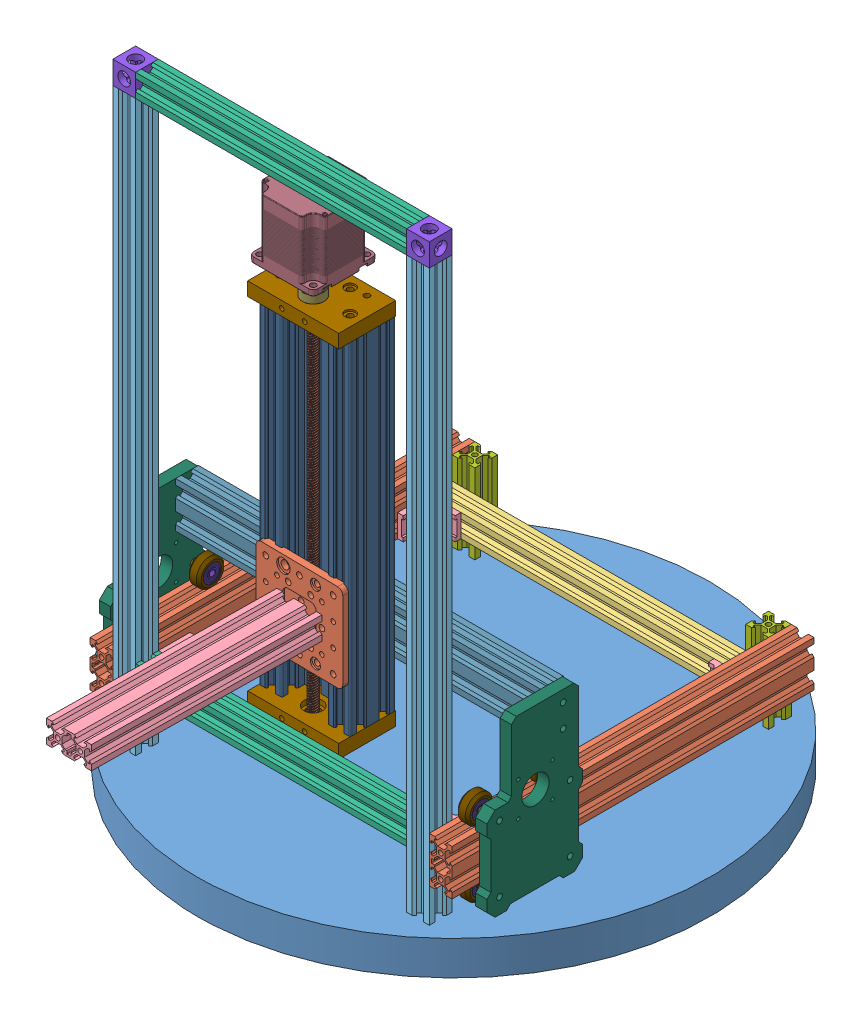
SolidWorks assembly Main, configuration Predeterminado. Lengths in mm.
Overall size (450 550 553.32).
74 component instances, 23 part files, 11 mates.
Components (placement in the parent):
- Base-1: Base [Predeterminado] at (-4.6545 -30.3598 450) size (450 30 450)
- XFrame-1: XFrame [Predeterminado] at (-136.0419 47.8198 132.7398) x (1 0 -0.000004) z (0.000004 0 1) size (318 520 318)
  - XBosch2040-1: XBosch2040 [Predeterminado] at (-28.3648 1.8204 159) size (20 40 318)
  - XBosch2020-3: XBosch2020 [Predeterminado] at (-8.3648 1.8204 457) x (0 0 -1) z (1 0 0) size (20 20 278)
  - XBosch2040-3: XBosch2040 [Predeterminado] at (269.6352 1.8204 159) size (20 40 318)
  - XBosch2020-4: XBosch2020 [Predeterminado] at (-8.3648 1.8204 199) x (0 0 -1) z (1 0 0) size (20 20 278)
  - 20X28.step-1: 20X28.step [Predeterminado] at (-8.3648 -8.1796 423.1) x (0 1 0) z (1 0 0) size (20 29.3 29.3)
  - 20X28.step-2: 20X28.step [Predeterminado] at (255.7352 -8.1796 437) x (0 1 0) z (0 0 -1) size (20 29.3 29.3)
  - 20X28.step-5: 20X28.step [Predeterminado] at (269.6352 -8.1796 212.9) x (0 1 0) z (-1 0 0) size (20 29.3 29.3)
  - 20X28.step-6: 20X28.step [Predeterminado] at (-8.3648 -8.1796 212.9) x (0 -1 0) z (1 0 0) size (20 29.3 29.3)
  - BaseKinectBosch2020-1: BaseKinectBosch2020 [Predeterminado] at (249.6352 -48.1796 477) x (0 0 -1) z (0 1 0) size (20 20 500)
  - BaseKinectBosch2020-3: BaseKinectBosch2020 [Predeterminado] at (-8.3648 -48.1796 477) x (0 0 -1) z (0 1 0) size (20 20 500)
  - SupportKinectBosch2020-2: SupportKinectBosch2020 [Predeterminado] at (11.6352 21.8204 477) x (0 0 -1) z (1 0 0) size (20 20 238)
  - SupportKinectBosch2020-3: SupportKinectBosch2020 [Predeterminado] at (11.6352 471.8204 477) x (0 0 -1) z (1 0 0) size (20 20 238)
  - SBaseKinectBosch2020-1: SBaseKinectBosch2020 [Predeterminado] at (-8.3648 21.8204 179) x (1 0 0) z (0 -1 0) size (20 20 70)
  - SBaseKinectBosch2020-2: SBaseKinectBosch2020 [Predeterminado] at (249.6352 21.8204 179) x (1 0 0) z (0 -1 0) size (20 20 70)
  - 2020CubeConnector.stp-1: 2020CubeConnector.stp [Predeterminado] at (-8.3648 451.8204 477) size (20 20 20)
  - 2020CubeConnector.stp-2: 2020CubeConnector.stp [Predeterminado] at (269.6352 451.8204 477) x (0 0 -1) z (1 0 0) size (20 20 20)
- LinearActuator-1: LinearActuator [Predeterminado] at (-0.8488 42.2282 481.3447) x (1 0 -0.000004) z (0.000004 0 1) size (80 409.44 60.6)
  - C-BeamEnd-2: C-BeamEnd [Predeterminado] at (-11.3983 29.7078 77.0996) x (1 0 0) z (0 0 -1) size (80 12 50)
  - C-Beam300-2: C-Beam300 [Predeterminado] at (-11.3983 329.7078 72.0996) x (-1 0 0) z (0 -1 0) size (80 40 300)
  - ScrewAxisZ-1: ScrewAxisZ [Default] at (-11.3983 17.7078 84.4996) x (0.069055 0 -0.997613) z (0 -1 0) size (8.33 8.33 405.47)
  - C-BeamEnd-3: C-BeamEnd [Predeterminado] at (-11.3983 329.7078 77.0996) x (-1 0 0) z (0 0 -1) size (80 12 50)
  - Coupler 6.35-8mm-1: Coupler 6.35-8mm [Default] at (-11.3983 354.2078 84.4996) x (0.045113 0 -0.998982) z (0 1 0) size (19.34 19.34 25)
  - Nema 23-1: Nema 23 [Default] at (-11.3983 424.3078 84.4996) x (-1 0 0) z (0 -1 0) size (56.4 59.4 76.6)
- YAxis-1: YAxis [Predeterminado] at (-525.5801 128.1994 508.9368) x (-0.000004 0 -1) z (1 0 -0.000004) size (90.84 144.12 340.6)
  - YBosch2040-1: YBosch2040 [Predeterminado] at (-24.5098 3.6408 360) size (20 40 320.6)
  - AxisY-Carrier-1: AxisY-Carrier [Predeterminado] at (-39.5098 -77.3592 350) size (84.07 143.54 10)
  - AxisY-Carrier-2: AxisY-Carrier [Predeterminado] at (-39.5098 -77.3592 680.6) size (84.07 143.54 10)
  - INSERTO_M5x0,8x6-2: INSERTO_M5x0,8x6 [Valor predeterminado] at (-70.5098 -48.3592 360) x (0.849028 0.528347 0) z (0.528347 -0.849028 0) size (7 6.95 6.99)
  - INSERTO_M5x0,8x6-3: INSERTO_M5x0,8x6 [Valor predeterminado] at (-8.5098 -48.3592 360) x (0 1 0) z (1 0 0) size (7 6.95 6.99)
  - INSERTO_M5x0,8x6-4: INSERTO_M5x0,8x6 [Valor predeterminado] at (-70.5098 -106.3592 360) x (0 1 0) z (1 0 0) size (7 6.95 6.99)
  - INSERTO_M5x0,8x6-5: INSERTO_M5x0,8x6 [Valor predeterminado] at (-8.5098 -106.3592 360) x (0 1 0) z (1 0 0) size (7 6.95 6.99)
  - INSERTO_M5x0,8x6-6: INSERTO_M5x0,8x6 [Valor predeterminado] at (-8.5098 -48.3592 674.6) x (0 1 0) z (1 0 0) size (7 6.95 6.99)
  - INSERTO_M5x0,8x6-7: INSERTO_M5x0,8x6 [Valor predeterminado] at (-70.5098 -48.3592 674.6) x (0.840532 0.541762 0) z (0.541762 -0.840532 0) size (7 6.95 6.99)
  - INSERTO_M5x0,8x6-8: INSERTO_M5x0,8x6 [Valor predeterminado] at (-8.5098 -106.3592 674.6) x (0 1 0) z (1 0 0) size (7 6.95 6.99)
  - INSERTO_M5x0,8x6-9: INSERTO_M5x0,8x6 [Valor predeterminado] at (-70.5098 -106.3592 674.6) x (0 1 0) z (1 0 0) size (7 6.95 6.99)
  - nylon-pulley-wheel-625zz.step-1: nylon-pulley-wheel-625zz.step [Predeterminado] at (-70.5098 -106.3592 669.4) x (0 0 -1) z (-0.999997 0.00242 0) size (10.4 24 24)
    - SKF_625_2Z v1.step-1: SKF_625_2Z v1.step [Predeterminado] at (-5.2 0 0) size (5 16 16)
    - Roldana V Nylon.step-1: Roldana V Nylon.step [Predeterminado] at origin size (10.4 24 24)
    - SKF_625_2Z v1 (1).step-1: SKF_625_2Z v1 (1).step [Predeterminado] at (5.2 0 0) x (-1 0 0) z (0 0 1) size (5 16 16)
  - nylon-pulley-wheel-625zz.step-2: nylon-pulley-wheel-625zz.step [Predeterminado] at (-70.5098 -48.3592 669.4) x (0 0 -1) z (1 0 0) size (10.4 24 24)
    - SKF_625_2Z v1.step-1: SKF_625_2Z v1.step [Predeterminado] at (-5.2 0 0) size (5 16 16)
    - Roldana V Nylon.step-1: Roldana V Nylon.step [Predeterminado] at origin size (10.4 24 24)
    - SKF_625_2Z v1 (1).step-1: SKF_625_2Z v1 (1).step [Predeterminado] at (5.2 0 0) x (-1 0 0) z (0 0 1) size (5 16 16)
  - nylon-pulley-wheel-625zz.step-3: nylon-pulley-wheel-625zz.step [Predeterminado] at (-8.5098 -48.3592 669.4) x (0 0 -1) z (0.968642 0.248459 0) size (10.4 24 24)
    - SKF_625_2Z v1.step-1: SKF_625_2Z v1.step [Predeterminado] at (-5.2 0 0) size (5 16 16)
    - Roldana V Nylon.step-1: Roldana V Nylon.step [Predeterminado] at origin size (10.4 24 24)
    - SKF_625_2Z v1 (1).step-1: SKF_625_2Z v1 (1).step [Predeterminado] at (5.2 0 0) x (-1 0 0) z (0 0 1) size (5 16 16)
  - nylon-pulley-wheel-625zz.step-4: nylon-pulley-wheel-625zz.step [Predeterminado] at (-8.5098 -106.3592 669.4) x (0 0 -1) z (0.999938 -0.011103 0) size (10.4 24 24)
    - SKF_625_2Z v1.step-1: SKF_625_2Z v1.step [Predeterminado] at (-5.2 0 0) size (5 16 16)
    - Roldana V Nylon.step-1: Roldana V Nylon.step [Predeterminado] at origin size (10.4 24 24)
    - SKF_625_2Z v1 (1).step-1: SKF_625_2Z v1 (1).step [Predeterminado] at (5.2 0 0) x (-1 0 0) z (0 0 1) size (5 16 16)
  - nylon-pulley-wheel-625zz.step-5: nylon-pulley-wheel-625zz.step [Predeterminado] at (-8.5098 -106.3592 371.2) x (0 0 -1) z (1 0 0) size (10.4 24 24)
    - SKF_625_2Z v1.step-1: SKF_625_2Z v1.step [Predeterminado] at (-5.2 0 0) size (5 16 16)
    - Roldana V Nylon.step-1: Roldana V Nylon.step [Predeterminado] at origin size (10.4 24 24)
    - SKF_625_2Z v1 (1).step-1: SKF_625_2Z v1 (1).step [Predeterminado] at (5.2 0 0) x (-1 0 0) z (0 0 1) size (5 16 16)
  - nylon-pulley-wheel-625zz.step-6: nylon-pulley-wheel-625zz.step [Predeterminado] at (-70.5098 -106.3592 371.2) x (0 0 -1) z (0.980573 0.196154 0) size (10.4 24 24)
    - SKF_625_2Z v1.step-1: SKF_625_2Z v1.step [Predeterminado] at (-5.2 0 0) size (5 16 16)
    - Roldana V Nylon.step-1: Roldana V Nylon.step [Predeterminado] at origin size (10.4 24 24)
    - SKF_625_2Z v1 (1).step-1: SKF_625_2Z v1 (1).step [Predeterminado] at (5.2 0 0) x (-1 0 0) z (0 0 1) size (5 16 16)
  - nylon-pulley-wheel-625zz.step-7: nylon-pulley-wheel-625zz.step [Predeterminado] at (-70.5098 -48.3592 371.2) x (0 0 -1) z (1 0 0) size (10.4 24 24)
    - SKF_625_2Z v1.step-1: SKF_625_2Z v1.step [Predeterminado] at (-5.2 0 0) size (5 16 16)
    - Roldana V Nylon.step-1: Roldana V Nylon.step [Predeterminado] at origin size (10.4 24 24)
    - SKF_625_2Z v1 (1).step-1: SKF_625_2Z v1 (1).step [Predeterminado] at (5.2 0 0) x (-1 0 0) z (0 0 1) size (5 16 16)
  - nylon-pulley-wheel-625zz.step-8: nylon-pulley-wheel-625zz.step [Predeterminado] at (-8.5098 -48.3592 371.2) x (0 0 -1) z (0.965283 -0.261208 0) size (10.4 24 24)
    - SKF_625_2Z v1.step-1: SKF_625_2Z v1.step [Predeterminado] at (-5.2 0 0) size (5 16 16)
    - Roldana V Nylon.step-1: Roldana V Nylon.step [Predeterminado] at origin size (10.4 24 24)
    - SKF_625_2Z v1 (1).step-1: SKF_625_2Z v1 (1).step [Predeterminado] at (5.2 0 0) x (-1 0 0) z (0 0 1) size (5 16 16)
- Arm-1: Arm [Predeterminado] at (-11.8566 145.5398 494.6935) x (0.999919 0 0.012739) z (-0.012739 0 0.999919) size (77.15 77.15 218)
  - C-BeamPlate-1: C-BeamPlate [Predeterminado] at (0.5163 1.4458 77.15) x (0 1 0) z (0 0 1) size (77.15 77.15 6)
  - Anti-BacklashBlock-1: Anti-BacklashBlock [Predeterminado] at (0.5163 -2.0542 65.15) x (0 -1 0) z (-1 0 0) size (33 12 34)
  - ZBosch2040-1: ZBosch2040 [Predeterminado] at (0.5163 11.4458 83.15) x (0 -1 0) z (0 0 1) size (20 40 200)
- CilinderForY-1: CilinderForY [Predeterminado] at (-159.5796 59.5227 607.7399) x (-0.000002 -0.902624 -0.43043) z (1 0 -0.000004) size (4 4 1.35)
Mates (geometry in assembly coordinates):
- Bloquear1: lock: unknown of Base-1; unknown of XFrame-1/XBosch2020-1
- Coincidente1: coincident anti-aligned: plane of LinearActuator-1/C-Beam300-2 through (-17.6668 371.936 533.4444) normal (-0.000004 0 -1); plane of YAxis-1/YBosch2040-1 through (155.02 131.8402 533.4436) normal (0.000004 0 1)
- Concéntrica1: concentric anti-aligned: cylinder of LinearActuator-1/C-BeamEnd-2 through (-12.2467 71.936 565.8443) axis (0 1 0) radius 8.05; cylinder of Arm-1/Anti-BacklashBlock-1 through (-12.2467 139.9855 565.8443) axis (0 -1 0) radius 3.3235
- Coincidente2: coincident anti-aligned: plane of Base-1 through (-4.6545 -0.3598 450) normal (0 1 0); plane of XFrame-1/BaseKinectBosch2020-1 through (113.5954 -0.3598 609.7388) normal (0 -1 0)
- Bloquear2: lock: unknown of Base-1; unknown of XFrame-1/XBosch2040-3
- Tangente3: tangent aligned: plane of XFrame-1/XBosch2040-1 through (-164.4046 67.8402 609.74) normal (0 -1 0); cylinder of YAxis-1/nylon-pulley-wheel-625zz.step-7/Roldana V Nylon.step-1 through (-154.3798 79.8402 579.445) axis (1 0 -0.000004) radius 12
- Tangente4: tangent aligned: plane of XFrame-1/XBosch2040-1 through (-164.4046 67.8402 609.74) normal (0 -1 0); cylinder of YAxis-1/nylon-pulley-wheel-625zz.step-8/Roldana V Nylon.step-1 through (-154.38 79.8402 517.445) axis (1 0 -0.000004) radius 12
- Coincidente4: coincident anti-aligned: plane of XFrame-1/XBosch2040-1 through (-158.2296 49.6402 609.7399) normal (-1 0 0.000004); plane of CilinderForY-1 through (-158.2296 59.5227 607.7399) normal (1 0 -0.000004)
- Tangente5: tangent aligned: plane of XFrame-1/XBosch2040-1 through (-164.4046 49.6402 609.74) normal (0.000004 0 1); cylinder of CilinderForY-1 through (-158.2296 59.5227 607.7399) axis (-1 0 0.000004) radius 2
- Bloquear5: lock: unknown of XFrame-1/XBosch2040-1; unknown of CilinderForY-1
- Coincidente10: coincident aligned: plane of YAxis-1/nylon-pulley-wheel-625zz.step-7/Roldana V Nylon.step-1 through (-159.5798 79.8402 569.645) normal (-1 0 0.000004); plane of CilinderForY-1 through (-159.5796 59.5227 607.7399) normal (-1 0 0.000004)
